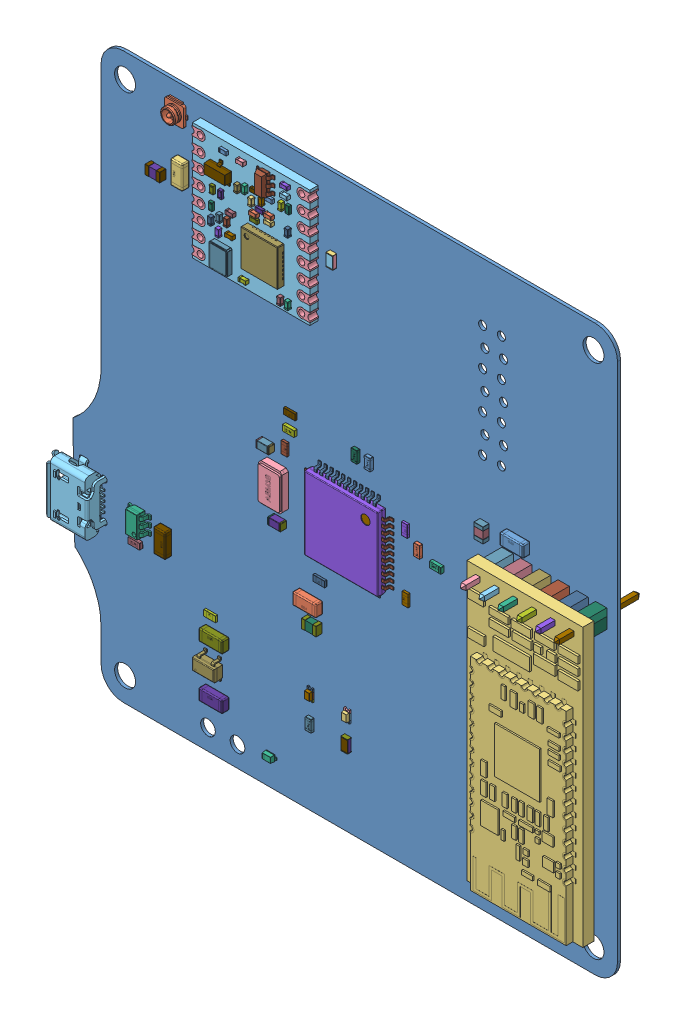
SolidWorks assembly Печатная плата Peggy Receiver, configuration Default. Lengths in mm.
Overall size (75.31 78.06 11.44).
265 component instances, 108 part files, 0 mates.
Components (placement in the parent):
- Печатная плата Peggy Receiver(2)^Печатная плата Peggy Receiver-2: Печатная плата Peggy Receiver(2)^Печатная плата Peggy Receiver [Default] at origin size (75.31 78.06 11.44) (virtual)
  - Board^Печатная плата Peggy Receiver(2)_Печатная плата Peggy Receiver-2: Board^Печатная плата Peggy Receiver(2)_Печатная плата Peggy Receiver [Default] at origin size (73.81 76.5 0.41) (virtual)
    - Open CASCADE STEP translator 7.5 1.1.1^Board_Печатная плата Peggy Receiver(2)_Печатная плата Peggy Receiver-1: Open CASCADE STEP translator 7.5 1.1.1^Board_Печатная плата Peggy Receiver(2)_Печатная плата Peggy Receiver [Default] at (0 0 -0.4115) size (73.81 76.5 0.41) (virtual)
  - XW1^Печатная плата Peggy Receiver(2)_Печатная плата Peggy Receiver-2: XW1^Печатная плата Peggy Receiver(2)_Печатная плата Peggy Receiver [Default] at origin size (3.01 2.86 1.29) (virtual)
    - IPX^XW1_Печатная плата Peggy Receiver(2)_Печатная плата Peggy Receiver-1: IPX^XW1_Печатная плата Peggy Receiver(2)_Печатная плата Peggy Receiver [Default] at (14.0624 73.0251 1.27) x (0 1 0) z (0 0 1) size (3.01 2.86 1.29) (virtual)
  - D1^Печатная плата Peggy Receiver(2)_Печатная плата Peggy Receiver-2: D1^Печатная плата Peggy Receiver(2)_Печатная плата Peggy Receiver [Default] at origin size (15.7 37.6 11.44) (virtual)
    - HC-SERIES^D1_Печатная плата Peggy Receiver(2)_Печатная плата Peggy Receiver-1: HC-SERIES^D1_Печатная плата Peggy Receiver(2)_Печатная плата Peggy Receiver [Default] at (65.255 43.965 4) x (0 -1 0) z (-1 0 0) size (37.6 11.44 15.7) (virtual)
      - HC-SERIES.stp^HC-SERIES_D1_Печатная плата Peggy Receiver(2)_Печатная плата Peggy Receiver-1: HC-SERIES.stp^HC-SERIES_D1_Печатная плата Peggy Receiver(2)_Печатная плата Peggy Receiver [Default] at origin size (37.6 11.44 15.7) (virtual)
        - Assembly1.stp^HC-SERIES.stp_HC-SERIES_D1_Печатная плата Peggy Receiver(2)_Печатная плата Peggy Receiver-1: Assembly1.stp^HC-SERIES.stp_HC-SERIES_D1_Печатная плата Peggy Receiver(2)_Печатная плата Peggy Receiver [Default] at origin size (37.6 2.6 15.7) (virtual)
          - _______-________9.stp^Assembly1.stp_HC-SERIES.stp_HC-SERIES_D1_Печатная плата Peggy Receiver(2)_Печатная плата Peggy Receiver-1: _______-________9.stp^Assembly1.stp_HC-SERIES.stp_HC-SERIES_D1_Печатная плата Peggy Receiver(2)_Печатная плата Peggy Receiver [Default] at origin size (37.6 2.6 15.7) (virtual)
        - Assembly8.stp^HC-SERIES.stp_HC-SERIES_D1_Печатная плата Peggy Receiver(2)_Печатная плата Peggy Receiver-1: Assembly8.stp^HC-SERIES.stp_HC-SERIES_D1_Печатная плата Peggy Receiver(2)_Печатная плата Peggy Receiver [Default] at origin size (2.54 11.44 15.24) (virtual)
          - Pin Header 6 x 1 TH 2.54mm Pitch.stp^Assembly8.stp_HC-SERIES.stp_HC-SERIES_D1_Печатная плата Peggy Receiver(2)_Печатная плата Peggy Receiver-1: Pin Header 6 x 1 TH 2.54mm Pitch.stp^Assembly8.stp_HC-SERIES.stp_HC-SERIES_D1_Печатная плата Peggy Receiver(2)_Печатная плата Peggy Receiver [Default] at (1.3634 -4.0367 -6.3335) x (1 0 0) z (0 -1 0) size (0.64 0.64 11.43) (virtual)
          - Pin Header 6 x 1 TH 2.54mm Pitch-0.stp^Assembly8.stp_HC-SERIES.stp_HC-SERIES_D1_Печатная плата Peggy Receiver(2)_Печатная плата Peggy Receiver-1: Pin Header 6 x 1 TH 2.54mm Pitch-0.stp^Assembly8.stp_HC-SERIES.stp_HC-SERIES_D1_Печатная плата Peggy Receiver(2)_Печатная плата Peggy Receiver [Default] at (1.3634 -4.0367 -6.3335) x (1 0 0) z (0 -1 0) size (0.64 0.64 11.43) (virtual)
          - Pin Header 6 x 1 TH 2.54mm Pitch-1.stp^Assembly8.stp_HC-SERIES.stp_HC-SERIES_D1_Печатная плата Peggy Receiver(2)_Печатная плата Peggy Receiver-1: Pin Header 6 x 1 TH 2.54mm Pitch-1.stp^Assembly8.stp_HC-SERIES.stp_HC-SERIES_D1_Печатная плата Peggy Receiver(2)_Печатная плата Peggy Receiver [Default] at (1.3634 -4.0414 -6.3335) x (1 0 0) z (0 -1 0) size (0.64 0.64 11.43) (virtual)
          - Pin Header 6 x 1 TH 2.54mm Pitch-2.stp^Assembly8.stp_HC-SERIES.stp_HC-SERIES_D1_Печатная плата Peggy Receiver(2)_Печатная плата Peggy Receiver-1: Pin Header 6 x 1 TH 2.54mm Pitch-2.stp^Assembly8.stp_HC-SERIES.stp_HC-SERIES_D1_Печатная плата Peggy Receiver(2)_Печатная плата Peggy Receiver [Default] at (1.3634 -4.0354 -6.3335) x (1 0 0) z (0 -1 0) size (0.64 0.64 11.43) (virtual)
          - Pin Header 6 x 1 TH 2.54mm Pitch-3.stp^Assembly8.stp_HC-SERIES.stp_HC-SERIES_D1_Печатная плата Peggy Receiver(2)_Печатная плата Peggy Receiver-1: Pin Header 6 x 1 TH 2.54mm Pitch-3.stp^Assembly8.stp_HC-SERIES.stp_HC-SERIES_D1_Печатная плата Peggy Receiver(2)_Печатная плата Peggy Receiver [Default] at (1.3634 -4.0354 -6.3335) x (1 0 0) z (0 -1 0) size (0.64 0.63 11.43) (virtual)
          - Pin Header 6 x 1 TH 2.54mm Pitch-4.stp^Assembly8.stp_HC-SERIES.stp_HC-SERIES_D1_Печатная плата Peggy Receiver(2)_Печатная плата Peggy Receiver-1: Pin Header 6 x 1 TH 2.54mm Pitch-4.stp^Assembly8.stp_HC-SERIES.stp_HC-SERIES_D1_Печатная плата Peggy Receiver(2)_Печатная плата Peggy Receiver [Default] at (1.3634 -4.0354 -6.3335) x (1 0 0) z (0 -1 0) size (0.64 0.64 11.43) (virtual)
          - Pin Header 6 x 1 TH 2.54mm Pitch-5.stp^Assembly8.stp_HC-SERIES.stp_HC-SERIES_D1_Печатная плата Peggy Receiver(2)_Печатная плата Peggy Receiver-1: Pin Header 6 x 1 TH 2.54mm Pitch-5.stp^Assembly8.stp_HC-SERIES.stp_HC-SERIES_D1_Печатная плата Peggy Receiver(2)_Печатная плата Peggy Receiver [Default] at (1.3634 -1.5 -6.3335) x (1 0 0) z (0 -1 0) size (2.54 2.54 2.54) (virtual)
          - Pin Header 6 x 1 TH 2.54mm Pitch-6.stp^Assembly8.stp_HC-SERIES.stp_HC-SERIES_D1_Печатная плата Peggy Receiver(2)_Печатная плата Peggy Receiver-1: Pin Header 6 x 1 TH 2.54mm Pitch-6.stp^Assembly8.stp_HC-SERIES.stp_HC-SERIES_D1_Печатная плата Peggy Receiver(2)_Печатная плата Peggy Receiver [Default] at (1.3634 -1.5 -6.3335) x (1 0 0) z (0 -1 0) size (2.54 2.54 2.54) (virtual)
          - Pin Header 6 x 1 TH 2.54mm Pitch-7.stp^Assembly8.stp_HC-SERIES.stp_HC-SERIES_D1_Печатная плата Peggy Receiver(2)_Печатная плата Peggy Receiver-1: Pin Header 6 x 1 TH 2.54mm Pitch-7.stp^Assembly8.stp_HC-SERIES.stp_HC-SERIES_D1_Печатная плата Peggy Receiver(2)_Печатная плата Peggy Receiver [Default] at (1.3634 -1.5 -6.3335) x (1 0 0) z (0 -1 0) size (2.54 2.54 2.54) (virtual)
          - Pin Header 6 x 1 TH 2.54mm Pitch-8.stp^Assembly8.stp_HC-SERIES.stp_HC-SERIES_D1_Печатная плата Peggy Receiver(2)_Печатная плата Peggy Receiver-1: Pin Header 6 x 1 TH 2.54mm Pitch-8.stp^Assembly8.stp_HC-SERIES.stp_HC-SERIES_D1_Печатная плата Peggy Receiver(2)_Печатная плата Peggy Receiver [Default] at (1.3634 -1.5 -6.3335) x (1 0 0) z (0 -1 0) size (2.54 2.54 2.54) (virtual)
          - Pin Header 6 x 1 TH 2.54mm Pitch-9.stp^Assembly8.stp_HC-SERIES.stp_HC-SERIES_D1_Печатная плата Peggy Receiver(2)_Печатная плата Peggy Receiver-1: Pin Header 6 x 1 TH 2.54mm Pitch-9.stp^Assembly8.stp_HC-SERIES.stp_HC-SERIES_D1_Печатная плата Peggy Receiver(2)_Печатная плата Peggy Receiver [Default] at (1.3634 -1.5 -6.3335) x (1 0 0) z (0 -1 0) size (2.54 2.54 2.54) (virtual)
          - Pin Header 6 x 1 TH 2.54mm Pitch-10.stp^Assembly8.stp_HC-SERIES.stp_HC-SERIES_D1_Печатная плата Peggy Receiver(2)_Печатная плата Peggy Receiver-1: Pin Header 6 x 1 TH 2.54mm Pitch-10.stp^Assembly8.stp_HC-SERIES.stp_HC-SERIES_D1_Печатная плата Peggy Receiver(2)_Печатная плата Peggy Receiver [Default] at (1.3634 -1.5 -6.3335) x (1 0 0) z (0 -1 0) size (2.54 2.54 2.54) (virtual)
  - C13^Печатная плата Peggy Receiver(2)_Печатная плата Peggy Receiver-2: C13^Печатная плата Peggy Receiver(2)_Печатная плата Peggy Receiver [Default] at origin size (3.2 1.6 1) (virtual)
    - SW3dPS-1206 SMD Capacitor^C13_Печатная плата Peggy Receiver(2)_Печатная плата Peggy Receiver-1: SW3dPS-1206 SMD Capacitor^C13_Печатная плата Peggy Receiver(2)_Печатная плата Peggy Receiver [Default] at (19.609 14.0729 0) x (1 0 0) z (0 -1 0) size (3.2 1 1.6) (virtual)
  - C12^Печатная плата Peggy Receiver(2)_Печатная плата Peggy Receiver-2: C12^Печатная плата Peggy Receiver(2)_Печатная плата Peggy Receiver [Default] at origin size (3.2 1.6 1) (virtual)
    - SW3dPS-1206 SMD Capacitor^C12_Печатная плата Peggy Receiver(2)_Печатная плата Peggy Receiver-1: SW3dPS-1206 SMD Capacitor^C12_Печатная плата Peggy Receiver(2)_Печатная плата Peggy Receiver [Default] at (19.609 7.0729 0) x (1 0 0) z (0 -1 0) size (3.2 1 1.6) (virtual)
  - C11^Печатная плата Peggy Receiver(2)_Печатная плата Peggy Receiver-2: C11^Печатная плата Peggy Receiver(2)_Печатная плата Peggy Receiver [Default] at origin size (1.6 3.2 1) (virtual)
    - SW3dPS-1206 SMD Capacitor^C11_Печатная плата Peggy Receiver(2)_Печатная плата Peggy Receiver-1: SW3dPS-1206 SMD Capacitor^C11_Печатная плата Peggy Receiver(2)_Печатная плата Peggy Receiver [Default] at (12.6729 22.091 0) x (0 -1 0) z (-1 0 0) size (3.2 1 1.6) (virtual)
  - C6^Печатная плата Peggy Receiver(2)_Печатная плата Peggy Receiver-2: C6^Печатная плата Peggy Receiver(2)_Печатная плата Peggy Receiver [Default] at origin size (3.2 1.6 1) (virtual)
    - SW3dPS-1206 SMD Capacitor^C6_Печатная плата Peggy Receiver(2)_Печатная плата Peggy Receiver-1: SW3dPS-1206 SMD Capacitor^C6_Печатная плата Peggy Receiver(2)_Печатная плата Peggy Receiver [Default] at (60.4 45.7 0) x (1 0 0) z (0 -1 0) size (3.2 1 1.6) (virtual)
  - C5^Печатная плата Peggy Receiver(2)_Печатная плата Peggy Receiver-2: C5^Печатная плата Peggy Receiver(2)_Печатная плата Peggy Receiver [Default] at origin size (3.2 1.6 1) (virtual)
    - SW3dPS-1206 SMD Capacitor^C5_Печатная плата Peggy Receiver(2)_Печатная плата Peggy Receiver-1: SW3dPS-1206 SMD Capacitor^C5_Печатная плата Peggy Receiver(2)_Печатная плата Peggy Receiver [Default] at (32.309 24.6729 0) x (-1 0 0) z (0 1 0) size (3.2 1 1.6) (virtual)
  - C4^Печатная плата Peggy Receiver(2)_Печатная плата Peggy Receiver-2: C4^Печатная плата Peggy Receiver(2)_Печатная плата Peggy Receiver [Default] at origin size (1.6 3.2 1) (virtual)
    - SW3dPS-1206 SMD Capacitor^C4_Печатная плата Peggy Receiver(2)_Печатная плата Peggy Receiver-1: SW3dPS-1206 SMD Capacitor^C4_Печатная плата Peggy Receiver(2)_Печатная плата Peggy Receiver [Default] at (15 66.5 0) x (0 1 0) z (1 0 0) size (3.2 1 1.6) (virtual)
  - ZQ1^Печатная плата Peggy Receiver(2)_Печатная плата Peggy Receiver-2: ZQ1^Печатная плата Peggy Receiver(2)_Печатная плата Peggy Receiver [Default] at origin size (3.18 5 1.11) (virtual)
    - ABM3B^ZQ1_Печатная плата Peggy Receiver(2)_Печатная плата Peggy Receiver-1: ABM3B^ZQ1_Печатная плата Peggy Receiver(2)_Печатная плата Peggy Receiver [Default] at (27.6091 36.0728 0) x (0 1 0) z (1 0 0) size (5 1.11 3.17) (virtual)
  - X2^Печатная плата Peggy Receiver(2)_Печатная плата Peggy Receiver-2: X2^Печатная плата Peggy Receiver(2)_Печатная плата Peggy Receiver [Default] at origin size (5.43 8.2 3.3) (virtual)
    - User Library-MicroUSB-B_Molex_105017-0001^X2_Печатная плата Peggy Receiver(2)_Печатная плата Peggy Receiver-1: User Library-MicroUSB-B_Molex_105017-0001^X2_Печатная плата Peggy Receiver(2)_Печатная плата Peggy Receiver [Default] at (1.7 22.4 1.2) x (0 -1 0) z (-1 0 0) size (8.2 3.3 5.43) (virtual)
  - VD2^Печатная плата Peggy Receiver(2)_Печатная плата Peggy Receiver-2: VD2^Печатная плата Peggy Receiver(2)_Печатная плата Peggy Receiver [Default] at origin size (1.65 0.8 0.65) (virtual)
    - User Library-SOD523-2^VD2_Печатная плата Peggy Receiver(2)_Печатная плата Peggy Receiver-1: User Library-SOD523-2^VD2_Печатная плата Peggy Receiver(2)_Печатная плата Peggy Receiver [Default] at (26.8499 3.7999 0) x (0 1 0) z (1 0 0) size (0.8 0.65 1.65) (virtual)
  - VD1^Печатная плата Peggy Receiver(2)_Печатная плата Peggy Receiver-2: VD1^Печатная плата Peggy Receiver(2)_Печатная плата Peggy Receiver [Default] at origin size (0.81 1.61 0.61) (virtual)
    - User Library-LED_0603_R^VD1_Печатная плата Peggy Receiver(2)_Печатная плата Peggy Receiver-1: User Library-LED_0603_R^VD1_Печатная плата Peggy Receiver(2)_Печатная плата Peggy Receiver [Default] at (32.2999 13.773 0) x (0 1 0) z (0 0 1) size (1.61 0.81 0.61) (virtual)
      - User Library-LED_0603_R_Pocket002^User Library-LED_0603_R_VD1_Печатная плата Peggy Receiver(2)_Печатная плата Peggy Receiver-1: User Library-LED_0603_R_Pocket002^User Library-LED_0603_R_VD1_Печатная плата Peggy Receiver(2)_Печатная плата Peggy Receiver [Default] at origin size (0.41 0.81 0.21) (virtual)
      - User Library-LED_0603_R_Pad004^User Library-LED_0603_R_VD1_Печатная плата Peggy Receiver(2)_Печатная плата Peggy Receiver-1: User Library-LED_0603_R_Pad004^User Library-LED_0603_R_VD1_Печатная плата Peggy Receiver(2)_Печатная плата Peggy Receiver [Default] x (1 0 0) z (0 0 -1) size (0.4 0.8 0) (virtual)
      - User Library-LED_0603_R_Fillet^User Library-LED_0603_R_VD1_Печатная плата Peggy Receiver(2)_Печатная плата Peggy Receiver-1: User Library-LED_0603_R_Fillet^User Library-LED_0603_R_VD1_Печатная плата Peggy Receiver(2)_Печатная плата Peggy Receiver [Default] at origin size (1 0.7 0.4) (virtual)
      - User Library-LED_0603_R_Pocket001^User Library-LED_0603_R_VD1_Печатная плата Peggy Receiver(2)_Печатная плата Peggy Receiver-1: User Library-LED_0603_R_Pocket001^User Library-LED_0603_R_VD1_Печатная плата Peggy Receiver(2)_Печатная плата Peggy Receiver [Default] at origin size (0.4 0.8 0.2) (virtual)
      - User Library-LED_0603_R_Pad^User Library-LED_0603_R_VD1_Печатная плата Peggy Receiver(2)_Печатная плата Peggy Receiver-1: User Library-LED_0603_R_Pad^User Library-LED_0603_R_VD1_Печатная плата Peggy Receiver(2)_Печатная плата Peggy Receiver [Default] at origin size (0.8 0.8 0.2) (virtual)
  - U1^Печатная плата Peggy Receiver(2)_Печатная плата Peggy Receiver-2: U1^Печатная плата Peggy Receiver(2)_Печатная плата Peggy Receiver [Default] at origin size (3 2.8 1.4) (virtual)
    - AP2112K-3.3TRG1--3DModel-STEP-1^U1_Печатная плата Peggy Receiver(2)_Печатная плата Peggy Receiver-1: AP2112K-3.3TRG1--3DModel-STEP-1^U1_Печатная плата Peggy Receiver(2)_Печатная плата Peggy Receiver [Default] at (19.009 10.5729 0) x (-1 0 0) z (0 1 0) size (3 1.4 2.8) (virtual)
  - R9^Печатная плата Peggy Receiver(2)_Печатная плата Peggy Receiver-2: R9^Печатная плата Peggy Receiver(2)_Печатная плата Peggy Receiver [Default] at origin size (1.61 0.81 0.46) (virtual)
    - chip_0603_r^R9_Печатная плата Peggy Receiver(2)_Печатная плата Peggy Receiver-1: chip_0603_r^R9_Печатная плата Peggy Receiver(2)_Печатная плата Peggy Receiver [Default] at (9.4728 19.7911 0.21) x (0 1 0) z (0 0 1) size (0.81 1.61 0.46) (virtual)
  - R8^Печатная плата Peggy Receiver(2)_Печатная плата Peggy Receiver-2: R8^Печатная плата Peggy Receiver(2)_Печатная плата Peggy Receiver [Default] at origin size (0.81 1.61 0.46) (virtual)
    - chip_0603_r^R8_Печатная плата Peggy Receiver(2)_Печатная плата Peggy Receiver-1: chip_0603_r^R8_Печатная плата Peggy Receiver(2)_Печатная плата Peggy Receiver [Default] at (32.2999 11.0999 0.21) x (-1 0 0) z (0 0 1) size (0.81 1.61 0.46) (virtual)
  - R7^Печатная плата Peggy Receiver(2)_Печатная плата Peggy Receiver-2: R7^Печатная плата Peggy Receiver(2)_Печатная плата Peggy Receiver [Default] at origin size (0.81 1.61 0.46) (virtual)
    - chip_0603_r^R7_Печатная плата Peggy Receiver(2)_Печатная плата Peggy Receiver-1: chip_0603_r^R7_Печатная плата Peggy Receiver(2)_Печатная плата Peggy Receiver [Default] at (38.5089 45.7728 0.21) x (-1 0 0) z (0 0 1) size (0.81 1.61 0.46) (virtual)
  - R6^Печатная плата Peggy Receiver(2)_Печатная плата Peggy Receiver-2: R6^Печатная плата Peggy Receiver(2)_Печатная плата Peggy Receiver [Default] at origin size (0.9 1.7 0.55) (virtual)
    - 6665909488^R6_Печатная плата Peggy Receiver(2)_Печатная плата Peggy Receiver-1: 6665909488^R6_Печатная плата Peggy Receiver(2)_Печатная плата Peggy Receiver [Default] at (37.2999 10.5001 0) x (0 1 0) z (0 0 1) size (1.7 0.9 0.55) (virtual)
      - Terminal^6665909488_R6_Печатная плата Peggy Receiver(2)_Печатная плата Peggy Receiver-1: Terminal^6665909488_R6_Печатная плата Peggy Receiver(2)_Печатная плата Peggy Receiver [Default] at (-0.85 -0.45 0) size (0.1 0.9 0.55) (virtual)
        - Open CASCADE STEP translator 6.8 15.2.1^Terminal_6665909488_R6_Печатная плата Peggy Receiver(2)_Печатная плата Peggy Receiver-1: Open CASCADE STEP translator 6.8 15.2.1^Terminal_6665909488_R6_Печатная плата Peggy Receiver(2)_Печатная плата Peggy Receiver [Default] at origin size (0.1 0.9 0.55) (virtual)
      - Terminal^6665909488_R6_Печатная плата Peggy Receiver(2)_Печатная плата Peggy Receiver-2: Terminal^6665909488_R6_Печатная плата Peggy Receiver(2)_Печатная плата Peggy Receiver [Default] at (0.85 0.45 0) x (-1 0 0) z (0 0 1) size (0.1 0.9 0.55) (virtual)
        - Open CASCADE STEP translator 6.8 15.2.1^Terminal_6665909488_R6_Печатная плата Peggy Receiver(2)_Печатная плата Peggy Receiver-1: Open CASCADE STEP translator 6.8 15.2.1^Terminal_6665909488_R6_Печатная плата Peggy Receiver(2)_Печатная плата Peggy Receiver [Default] at origin size (0.1 0.9 0.55) (virtual)
      - Mid_Body^6665909488_R6_Печатная плата Peggy Receiver(2)_Печатная плата Peggy Receiver-1: Mid_Body^6665909488_R6_Печатная плата Peggy Receiver(2)_Печатная плата Peggy Receiver [Default] at (-0.85 -0.45 0) size (1.59 0.9 0.44) (virtual)
      - Mark^6665909488_R6_Печатная плата Peggy Receiver(2)_Печатная плата Peggy Receiver-1: Mark^6665909488_R6_Печатная плата Peggy Receiver(2)_Печатная плата Peggy Receiver [Default] at (-0.75 -0.45 0.495) size (1.5 0.9 0.06) (virtual)
  - R5^Печатная плата Peggy Receiver(2)_Печатная плата Peggy Receiver-2: R5^Печатная плата Peggy Receiver(2)_Печатная плата Peggy Receiver [Default] at origin size (0.81 1.61 0.46) (virtual)
    - chip_0603_r^R5_Печатная плата Peggy Receiver(2)_Печатная плата Peggy Receiver-1: chip_0603_r^R5_Печатная плата Peggy Receiver(2)_Печатная плата Peggy Receiver [Default] at (40.3089 45.7728 0.21) x (-1 0 0) z (0 0 1) size (0.81 1.61 0.46) (virtual)
  - R4^Печатная плата Peggy Receiver(2)_Печатная плата Peggy Receiver-2: R4^Печатная плата Peggy Receiver(2)_Печатная плата Peggy Receiver [Default] at origin size (0.81 1.61 0.46) (virtual)
    - chip_0603_r^R4_Печатная плата Peggy Receiver(2)_Печатная плата Peggy Receiver-1: chip_0603_r^R4_Печатная плата Peggy Receiver(2)_Печатная плата Peggy Receiver [Default] at (47.0089 38.8728 0.21) x (-1 0 0) z (0 0 1) size (0.81 1.61 0.46) (virtual)
  - R3^Печатная плата Peggy Receiver(2)_Печатная плата Peggy Receiver-2: R3^Печатная плата Peggy Receiver(2)_Печатная плата Peggy Receiver [Default] at origin size (0.9 1.7 0.55) (virtual)
    - 6665909808^R3_Печатная плата Peggy Receiver(2)_Печатная плата Peggy Receiver-1: 6665909808^R3_Печатная плата Peggy Receiver(2)_Печатная плата Peggy Receiver [Default] at (35.3001 66.2999 0) x (0 -1 0) z (0 0 1) size (1.7 0.9 0.55) (virtual)
      - Terminal-1^6665909808_R3_Печатная плата Peggy Receiver(2)_Печатная плата Peggy Receiver-1: Terminal-1^6665909808_R3_Печатная плата Peggy Receiver(2)_Печатная плата Peggy Receiver [Default] at (-0.85 -0.45 0) size (0.1 0.9 0.55) (virtual)
        - Open CASCADE STEP translator 6.8 15.2.1-0^Terminal-1_6665909808_R3_Печатная плата Peggy Receiver(2)_Печатная плата Peggy Receiver-1: Open CASCADE STEP translator 6.8 15.2.1-0^Terminal-1_6665909808_R3_Печатная плата Peggy Receiver(2)_Печатная плата Peggy Receiver [Default] at origin size (0.1 0.9 0.55) (virtual)
      - Terminal-1^6665909808_R3_Печатная плата Peggy Receiver(2)_Печатная плата Peggy Receiver-2: Terminal-1^6665909808_R3_Печатная плата Peggy Receiver(2)_Печатная плата Peggy Receiver [Default] at (0.85 0.45 0) x (-1 0 0) z (0 0 1) size (0.1 0.9 0.55) (virtual)
        - Open CASCADE STEP translator 6.8 15.2.1-0^Terminal-1_6665909808_R3_Печатная плата Peggy Receiver(2)_Печатная плата Peggy Receiver-1: Open CASCADE STEP translator 6.8 15.2.1-0^Terminal-1_6665909808_R3_Печатная плата Peggy Receiver(2)_Печатная плата Peggy Receiver [Default] at origin size (0.1 0.9 0.55) (virtual)
      - Mid_Body-1^6665909808_R3_Печатная плата Peggy Receiver(2)_Печатная плата Peggy Receiver-1: Mid_Body-1^6665909808_R3_Печатная плата Peggy Receiver(2)_Печатная плата Peggy Receiver [Default] at (-0.85 -0.45 0) size (1.59 0.9 0.44) (virtual)
      - Mark-2^6665909808_R3_Печатная плата Peggy Receiver(2)_Печатная плата Peggy Receiver-1: Mark-2^6665909808_R3_Печатная плата Peggy Receiver(2)_Печатная плата Peggy Receiver [Default] at (-0.75 -0.45 0.495) size (1.5 0.9 0.06) (virtual)
  - R2^Печатная плата Peggy Receiver(2)_Печатная плата Peggy Receiver-2: R2^Печатная плата Peggy Receiver(2)_Печатная плата Peggy Receiver [Default] at origin size (1.61 0.81 0.46) (virtual)
    - chip_0603_r^R2_Печатная плата Peggy Receiver(2)_Печатная плата Peggy Receiver-1: chip_0603_r^R2_Печатная плата Peggy Receiver(2)_Печатная плата Peggy Receiver [Default] at (48.7091 37.3728 0.21) x (0 -1 0) z (0 0 1) size (0.81 1.61 0.46) (virtual)
  - R1^Печатная плата Peggy Receiver(2)_Печатная плата Peggy Receiver-2: R1^Печатная плата Peggy Receiver(2)_Печатная плата Peggy Receiver [Default] at origin size (1.61 0.81 0.46) (virtual)
    - chip_0603_r^R1_Печатная плата Peggy Receiver(2)_Печатная плата Peggy Receiver-1: chip_0603_r^R1_Печатная плата Peggy Receiver(2)_Печатная плата Peggy Receiver [Default] at (30.4089 43.473 0.21) x (0 1 0) z (0 0 1) size (0.81 1.61 0.46) (virtual)
  - MPU1^Печатная плата Peggy Receiver(2)_Печатная плата Peggy Receiver-2: MPU1^Печатная плата Peggy Receiver(2)_Печатная плата Peggy Receiver [Default] at origin size (14.96 12 1.2) (virtual)
    - 6665910048^MPU1_Печатная плата Peggy Receiver(2)_Печатная плата Peggy Receiver-1: 6665910048^MPU1_Печатная плата Peggy Receiver(2)_Печатная плата Peggy Receiver [Default] at (37.5091 35.7228 0) x (0 -1 0) z (0 0 1) size (12 14.96 1.2) (virtual)
      - Body^6665910048_MPU1_Печатная плата Peggy Receiver(2)_Печатная плата Peggy Receiver-1: Body^6665910048_MPU1_Печатная плата Peggy Receiver(2)_Печатная плата Peggy Receiver [Default] at (-5 -5 0) size (10.01 10.01 1.15) (virtual)
        - Open CASCADE STEP translator 6.8 62.2.1^Body_6665910048_MPU1_Печатная плата Peggy Receiver(2)_Печатная плата Peggy Receiver-1: Open CASCADE STEP translator 6.8 62.2.1^Body_6665910048_MPU1_Печатная плата Peggy Receiver(2)_Печатная плата Peggy Receiver [Default] at origin size (10.01 10.01 1.15) (virtual)
      - Open CASCADE STEP translator 6.8 62.1^6665910048_MPU1_Печатная плата Peggy Receiver(2)_Печатная плата Peggy Receiver-1: Open CASCADE STEP translator 6.8 62.1^6665910048_MPU1_Печатная плата Peggy Receiver(2)_Печатная плата Peggy Receiver [Default] at (-5 -5 0.001) size (1.26 1.26 0.01) (virtual)
      - Leader^6665910048_MPU1_Печатная плата Peggy Receiver(2)_Печатная плата Peggy Receiver-1: Leader^6665910048_MPU1_Печатная плата Peggy Receiver(2)_Печатная плата Peggy Receiver [Default] at (-5 -4 0) x (-1 0 0) z (0 0 1) size (1 0.38 0.68) (virtual)
      - Leader^6665910048_MPU1_Печатная плата Peggy Receiver(2)_Печатная плата Peggy Receiver-2: Leader^6665910048_MPU1_Печатная плата Peggy Receiver(2)_Печатная плата Peggy Receiver [Default] at (-5 -3.2 0) x (-1 0 0) z (0 0 1) size (1 0.38 0.68) (virtual)
      - Leader^6665910048_MPU1_Печатная плата Peggy Receiver(2)_Печатная плата Peggy Receiver-3: Leader^6665910048_MPU1_Печатная плата Peggy Receiver(2)_Печатная плата Peggy Receiver [Default] at (-5 -2.4 0) x (-1 0 0) z (0 0 1) size (1 0.38 0.68) (virtual)
      - Leader^6665910048_MPU1_Печатная плата Peggy Receiver(2)_Печатная плата Peggy Receiver-4: Leader^6665910048_MPU1_Печатная плата Peggy Receiver(2)_Печатная плата Peggy Receiver [Default] at (-5 -1.6 0) x (-1 0 0) z (0 0 1) size (1 0.38 0.68) (virtual)
      - Leader^6665910048_MPU1_Печатная плата Peggy Receiver(2)_Печатная плата Peggy Receiver-5: Leader^6665910048_MPU1_Печатная плата Peggy Receiver(2)_Печатная плата Peggy Receiver [Default] at (-5 -0.8 0) x (-1 0 0) z (0 0 1) size (1 0.38 0.68) (virtual)
      - Leader^6665910048_MPU1_Печатная плата Peggy Receiver(2)_Печатная плата Peggy Receiver-6: Leader^6665910048_MPU1_Печатная плата Peggy Receiver(2)_Печатная плата Peggy Receiver [Default] at (-5 0 0) x (-1 0 0) z (0 0 1) size (1 0.38 0.68) (virtual)
      - Leader^6665910048_MPU1_Печатная плата Peggy Receiver(2)_Печатная плата Peggy Receiver-7: Leader^6665910048_MPU1_Печатная плата Peggy Receiver(2)_Печатная плата Peggy Receiver [Default] at (-5 0.8 0) x (-1 0 0) z (0 0 1) size (1 0.38 0.68) (virtual)
      - Leader^6665910048_MPU1_Печатная плата Peggy Receiver(2)_Печатная плата Peggy Receiver-8: Leader^6665910048_MPU1_Печатная плата Peggy Receiver(2)_Печатная плата Peggy Receiver [Default] at (-5 1.6 0) x (-1 0 0) z (0 0 1) size (1 0.38 0.68) (virtual)
      - Leader^6665910048_MPU1_Печатная плата Peggy Receiver(2)_Печатная плата Peggy Receiver-9: Leader^6665910048_MPU1_Печатная плата Peggy Receiver(2)_Печатная плата Peggy Receiver [Default] at (-5 2.4 0) x (-1 0 0) z (0 0 1) size (1 0.38 0.68) (virtual)
      - Leader^6665910048_MPU1_Печатная плата Peggy Receiver(2)_Печатная плата Peggy Receiver-10: Leader^6665910048_MPU1_Печатная плата Peggy Receiver(2)_Печатная плата Peggy Receiver [Default] at (-5 3.2 0) x (-1 0 0) z (0 0 1) size (1 0.38 0.68) (virtual)
      - Leader^6665910048_MPU1_Печатная плата Peggy Receiver(2)_Печатная плата Peggy Receiver-11: Leader^6665910048_MPU1_Печатная плата Peggy Receiver(2)_Печатная плата Peggy Receiver [Default] at (-5 4 0) x (-1 0 0) z (0 0 1) size (1 0.38 0.68) (virtual)
      - Leader^6665910048_MPU1_Печатная плата Peggy Receiver(2)_Печатная плата Peggy Receiver-12: Leader^6665910048_MPU1_Печатная плата Peggy Receiver(2)_Печатная плата Peggy Receiver [Default] at (5 -4 0) size (1 0.38 0.68) (virtual)
      - Leader^6665910048_MPU1_Печатная плата Peggy Receiver(2)_Печатная плата Peggy Receiver-13: Leader^6665910048_MPU1_Печатная плата Peggy Receiver(2)_Печатная плата Peggy Receiver [Default] at (5 -3.2 0) size (1 0.38 0.68) (virtual)
      - Leader^6665910048_MPU1_Печатная плата Peggy Receiver(2)_Печатная плата Peggy Receiver-14: Leader^6665910048_MPU1_Печатная плата Peggy Receiver(2)_Печатная плата Peggy Receiver [Default] at (5 -2.4 0) size (1 0.38 0.68) (virtual)
      - Leader^6665910048_MPU1_Печатная плата Peggy Receiver(2)_Печатная плата Peggy Receiver-15: Leader^6665910048_MPU1_Печатная плата Peggy Receiver(2)_Печатная плата Peggy Receiver [Default] at (5 -1.6 0) size (1 0.38 0.68) (virtual)
      - Leader^6665910048_MPU1_Печатная плата Peggy Receiver(2)_Печатная плата Peggy Receiver-16: Leader^6665910048_MPU1_Печатная плата Peggy Receiver(2)_Печатная плата Peggy Receiver [Default] at (5 -0.8 0) size (1 0.38 0.68) (virtual)
      - Leader^6665910048_MPU1_Печатная плата Peggy Receiver(2)_Печатная плата Peggy Receiver-17: Leader^6665910048_MPU1_Печатная плата Peggy Receiver(2)_Печатная плата Peggy Receiver [Default] at (5 0 0) size (1 0.38 0.68) (virtual)
      - Leader^6665910048_MPU1_Печатная плата Peggy Receiver(2)_Печатная плата Peggy Receiver-18: Leader^6665910048_MPU1_Печатная плата Peggy Receiver(2)_Печатная плата Peggy Receiver [Default] at (5 0.8 0) size (1 0.38 0.68) (virtual)
      - Leader^6665910048_MPU1_Печатная плата Peggy Receiver(2)_Печатная плата Peggy Receiver-19: Leader^6665910048_MPU1_Печатная плата Peggy Receiver(2)_Печатная плата Peggy Receiver [Default] at (5 1.6 0) size (1 0.38 0.68) (virtual)
      - Leader^6665910048_MPU1_Печатная плата Peggy Receiver(2)_Печатная плата Peggy Receiver-20: Leader^6665910048_MPU1_Печатная плата Peggy Receiver(2)_Печатная плата Peggy Receiver [Default] at (5 2.4 0) size (1 0.38 0.68) (virtual)
      - Leader^6665910048_MPU1_Печатная плата Peggy Receiver(2)_Печатная плата Peggy Receiver-21: Leader^6665910048_MPU1_Печатная плата Peggy Receiver(2)_Печатная плата Peggy Receiver [Default] at (5 3.2 0) size (1 0.38 0.68) (virtual)
      - Leader^6665910048_MPU1_Печатная плата Peggy Receiver(2)_Печатная плата Peggy Receiver-22: Leader^6665910048_MPU1_Печатная плата Peggy Receiver(2)_Печатная плата Peggy Receiver [Default] at (5 4 0) size (1 0.38 0.68) (virtual)
      - Leader-3^6665910048_MPU1_Печатная плата Peggy Receiver(2)_Печатная плата Peggy Receiver-1: Leader-3^6665910048_MPU1_Печатная плата Peggy Receiver(2)_Печатная плата Peggy Receiver [Default] at (-4 -5 0) x (0 -1 0) z (0 0 1) size (1 0.38 0.68) (virtual)
      - Leader-3^6665910048_MPU1_Печатная плата Peggy Receiver(2)_Печатная плата Peggy Receiver-2: Leader-3^6665910048_MPU1_Печатная плата Peggy Receiver(2)_Печатная плата Peggy Receiver [Default] at (-3.2 -5 0) x (0 -1 0) z (0 0 1) size (1 0.38 0.68) (virtual)
      - Leader-3^6665910048_MPU1_Печатная плата Peggy Receiver(2)_Печатная плата Peggy Receiver-3: Leader-3^6665910048_MPU1_Печатная плата Peggy Receiver(2)_Печатная плата Peggy Receiver [Default] at (-2.4 -5 0) x (0 -1 0) z (0 0 1) size (1 0.38 0.68) (virtual)
      - Leader-3^6665910048_MPU1_Печатная плата Peggy Receiver(2)_Печатная плата Peggy Receiver-4: Leader-3^6665910048_MPU1_Печатная плата Peggy Receiver(2)_Печатная плата Peggy Receiver [Default] at (-1.6 -5 0) x (0 -1 0) z (0 0 1) size (1 0.38 0.68) (virtual)
      - Leader-3^6665910048_MPU1_Печатная плата Peggy Receiver(2)_Печатная плата Peggy Receiver-5: Leader-3^6665910048_MPU1_Печатная плата Peggy Receiver(2)_Печатная плата Peggy Receiver [Default] at (-0.8 -5 0) x (0 -1 0) z (0 0 1) size (1 0.38 0.68) (virtual)
      - Leader-3^6665910048_MPU1_Печатная плата Peggy Receiver(2)_Печатная плата Peggy Receiver-6: Leader-3^6665910048_MPU1_Печатная плата Peggy Receiver(2)_Печатная плата Peggy Receiver [Default] at (0 -5 0) x (0 -1 0) z (0 0 1) size (1 0.38 0.68) (virtual)
      - Leader-3^6665910048_MPU1_Печатная плата Peggy Receiver(2)_Печатная плата Peggy Receiver-7: Leader-3^6665910048_MPU1_Печатная плата Peggy Receiver(2)_Печатная плата Peggy Receiver [Default] at (0.8 -5 0) x (0 -1 0) z (0 0 1) size (1 0.38 0.68) (virtual)
      - Leader-3^6665910048_MPU1_Печатная плата Peggy Receiver(2)_Печатная плата Peggy Receiver-8: Leader-3^6665910048_MPU1_Печатная плата Peggy Receiver(2)_Печатная плата Peggy Receiver [Default] at (1.6 -5 0) x (0 -1 0) z (0 0 1) size (1 0.38 0.68) (virtual)
      - Leader-3^6665910048_MPU1_Печатная плата Peggy Receiver(2)_Печатная плата Peggy Receiver-9: Leader-3^6665910048_MPU1_Печатная плата Peggy Receiver(2)_Печатная плата Peggy Receiver [Default] at (2.4 -5 0) x (0 -1 0) z (0 0 1) size (1 0.38 0.68) (virtual)
      - Leader-3^6665910048_MPU1_Печатная плата Peggy Receiver(2)_Печатная плата Peggy Receiver-10: Leader-3^6665910048_MPU1_Печатная плата Peggy Receiver(2)_Печатная плата Peggy Receiver [Default] at (3.2 -5 0) x (0 -1 0) z (0 0 1) size (1 0.38 0.68) (virtual)
      - Leader-3^6665910048_MPU1_Печатная плата Peggy Receiver(2)_Печатная плата Peggy Receiver-11: Leader-3^6665910048_MPU1_Печатная плата Peggy Receiver(2)_Печатная плата Peggy Receiver [Default] at (4 -5 0) x (0 -1 0) z (0 0 1) size (1 0.38 0.68) (virtual)
      - Leader-3^6665910048_MPU1_Печатная плата Peggy Receiver(2)_Печатная плата Peggy Receiver-12: Leader-3^6665910048_MPU1_Печатная плата Peggy Receiver(2)_Печатная плата Peggy Receiver [Default] at (-4 5 0) x (0 1 0) z (0 0 1) size (1 0.38 0.68) (virtual)
      - Leader-3^6665910048_MPU1_Печатная плата Peggy Receiver(2)_Печатная плата Peggy Receiver-13: Leader-3^6665910048_MPU1_Печатная плата Peggy Receiver(2)_Печатная плата Peggy Receiver [Default] at (-3.2 5 0) x (0 1 0) z (0 0 1) size (1 0.38 0.68) (virtual)
      - Leader-3^6665910048_MPU1_Печатная плата Peggy Receiver(2)_Печатная плата Peggy Receiver-14: Leader-3^6665910048_MPU1_Печатная плата Peggy Receiver(2)_Печатная плата Peggy Receiver [Default] at (-2.4 5 0) x (0 1 0) z (0 0 1) size (1 0.38 0.68) (virtual)
      - Leader-3^6665910048_MPU1_Печатная плата Peggy Receiver(2)_Печатная плата Peggy Receiver-15: Leader-3^6665910048_MPU1_Печатная плата Peggy Receiver(2)_Печатная плата Peggy Receiver [Default] at (-1.6 5 0) x (0 1 0) z (0 0 1) size (1 0.38 0.68) (virtual)
      - Leader-3^6665910048_MPU1_Печатная плата Peggy Receiver(2)_Печатная плата Peggy Receiver-16: Leader-3^6665910048_MPU1_Печатная плата Peggy Receiver(2)_Печатная плата Peggy Receiver [Default] at (-0.8 5 0) x (0 1 0) z (0 0 1) size (1 0.38 0.68) (virtual)
      - Leader-3^6665910048_MPU1_Печатная плата Peggy Receiver(2)_Печатная плата Peggy Receiver-17: Leader-3^6665910048_MPU1_Печатная плата Peggy Receiver(2)_Печатная плата Peggy Receiver [Default] at (0 5 0) x (0 1 0) z (0 0 1) size (1 0.38 0.68) (virtual)
      - Leader-3^6665910048_MPU1_Печатная плата Peggy Receiver(2)_Печатная плата Peggy Receiver-18: Leader-3^6665910048_MPU1_Печатная плата Peggy Receiver(2)_Печатная плата Peggy Receiver [Default] at (0.8 5 0) x (0 1 0) z (0 0 1) size (1 0.38 0.68) (virtual)
      - Leader-3^6665910048_MPU1_Печатная плата Peggy Receiver(2)_Печатная плата Peggy Receiver-19: Leader-3^6665910048_MPU1_Печатная плата Peggy Receiver(2)_Печатная плата Peggy Receiver [Default] at (1.6 5 0) x (0 1 0) z (0 0 1) size (1 0.38 0.68) (virtual)
      - Leader-3^6665910048_MPU1_Печатная плата Peggy Receiver(2)_Печатная плата Peggy Receiver-20: Leader-3^6665910048_MPU1_Печатная плата Peggy Receiver(2)_Печатная плата Peggy Receiver [Default] at (2.4 5 0) x (0 1 0) z (0 0 1) size (1 0.38 0.68) (virtual)
      - Leader-3^6665910048_MPU1_Печатная плата Peggy Receiver(2)_Печатная плата Peggy Receiver-21: Leader-3^6665910048_MPU1_Печатная плата Peggy Receiver(2)_Печатная плата Peggy Receiver [Default] at (3.2 5 0) x (0 1 0) z (0 0 1) size (1 0.38 0.68) (virtual)
      - Leader-3^6665910048_MPU1_Печатная плата Peggy Receiver(2)_Печатная плата Peggy Receiver-22: Leader-3^6665910048_MPU1_Печатная плата Peggy Receiver(2)_Печатная плата Peggy Receiver [Default] at (4 5 0) x (0 1 0) z (0 0 1) size (1 0.38 0.68) (virtual)
    - User Library-VQFN(44)^MPU1_Печатная плата Peggy Receiver(2)_Печатная плата Peggy Receiver-1: User Library-VQFN(44)^MPU1_Печатная плата Peggy Receiver(2)_Печатная плата Peggy Receiver [Default] at (33.963 32.1998 0) x (1 0 0) z (0 -1 0) size (7.1 0.95 7.1) (virtual)
  - L3^Печатная плата Peggy Receiver(2)_Печатная плата Peggy Receiver-2: L3^Печатная плата Peggy Receiver(2)_Печатная плата Peggy Receiver [Default] at origin size (1.25 2 0.85) (virtual)
    - User Library-FB_2012-1^L3_Печатная плата Peggy Receiver(2)_Печатная плата Peggy Receiver-1: User Library-FB_2012-1^L3_Печатная плата Peggy Receiver(2)_Печатная плата Peggy Receiver [Default] at (55.7999 44.8001 0) x (0 1 0) z (0 0 1) size (2 1.25 0.85) (virtual)
      - User Library-FB_2012-1_Pad001^User Library-FB_2012-1_L3_Печатная плата Peggy Receiver(2)_Печатная плата Peggy Receiver-1: User Library-FB_2012-1_Pad001^User Library-FB_2012-1_L3_Печатная плата Peggy Receiver(2)_Печатная плата Peggy Receiver [Default] at (0 0 0.03) size (1.94 1.19 0.79) (virtual)
      - User Library-FB_2012-1_Cut^User Library-FB_2012-1_L3_Печатная плата Peggy Receiver(2)_Печатная плата Peggy Receiver-1: User Library-FB_2012-1_Cut^User Library-FB_2012-1_L3_Печатная плата Peggy Receiver(2)_Печатная плата Peggy Receiver [Default] at origin size (2 1.25 0.85) (virtual)
  - L2^Печатная плата Peggy Receiver(2)_Печатная плата Peggy Receiver-2: L2^Печатная плата Peggy Receiver(2)_Печатная плата Peggy Receiver [Default] at origin size (2 1.25 0.85) (virtual)
    - User Library-FB_2012-1^L2_Печатная плата Peggy Receiver(2)_Печатная плата Peggy Receiver-1: User Library-FB_2012-1^L2_Печатная плата Peggy Receiver(2)_Печатная плата Peggy Receiver [Default] at (32.8001 22.2001 0) x (1 0 0) z (0 0 1) size (2 1.25 0.85) (virtual)
      - User Library-FB_2012-1_Pad001^User Library-FB_2012-1_L2_Печатная плата Peggy Receiver(2)_Печатная плата Peggy Receiver-1: User Library-FB_2012-1_Pad001^User Library-FB_2012-1_L2_Печатная плата Peggy Receiver(2)_Печатная плата Peggy Receiver [Default] at (0 0 0.03) size (1.94 1.19 0.79) (virtual)
      - User Library-FB_2012-1_Cut^User Library-FB_2012-1_L2_Печатная плата Peggy Receiver(2)_Печатная плата Peggy Receiver-1: User Library-FB_2012-1_Cut^User Library-FB_2012-1_L2_Печатная плата Peggy Receiver(2)_Печатная плата Peggy Receiver [Default] at origin size (2 1.25 0.85) (virtual)
  - L1^Печатная плата Peggy Receiver(2)_Печатная плата Peggy Receiver-2: L1^Печатная плата Peggy Receiver(2)_Печатная плата Peggy Receiver [Default] at origin size (2 1.25 0.85) (virtual)
    - User Library-FB_2012-1^L1_Печатная плата Peggy Receiver(2)_Печатная плата Peggy Receiver-1: User Library-FB_2012-1^L1_Печатная плата Peggy Receiver(2)_Печатная плата Peggy Receiver [Default] at (11.5999 64.8999 0) x (-1 0 0) z (0 0 1) size (2 1.25 0.85) (virtual)
      - User Library-FB_2012-1_Pad001^User Library-FB_2012-1_L1_Печатная плата Peggy Receiver(2)_Печатная плата Peggy Receiver-1: User Library-FB_2012-1_Pad001^User Library-FB_2012-1_L1_Печатная плата Peggy Receiver(2)_Печатная плата Peggy Receiver [Default] at (0 0 0.03) size (1.94 1.19 0.79) (virtual)
      - User Library-FB_2012-1_Cut^User Library-FB_2012-1_L1_Печатная плата Peggy Receiver(2)_Печатная плата Peggy Receiver-1: User Library-FB_2012-1_Cut^User Library-FB_2012-1_L1_Печатная плата Peggy Receiver(2)_Печатная плата Peggy Receiver [Default] at origin size (2 1.25 0.85) (virtual)
  - HL1^Печатная плата Peggy Receiver(2)_Печатная плата Peggy Receiver-2: HL1^Печатная плата Peggy Receiver(2)_Печатная плата Peggy Receiver [Default] at origin size (0.81 1.61 0.61) (virtual)
    - User Library-LED_0603_G^HL1_Печатная плата Peggy Receiver(2)_Печатная плата Peggy Receiver-1: User Library-LED_0603_G^HL1_Печатная плата Peggy Receiver(2)_Печатная плата Peggy Receiver [Default] at (37.2999 13.773 0) x (0 1 0) z (0 0 1) size (1.61 0.81 0.61) (virtual)
      - User Library-LED_0603_G_Pocket002^User Library-LED_0603_G_HL1_Печатная плата Peggy Receiver(2)_Печатная плата Peggy Receiver-1: User Library-LED_0603_G_Pocket002^User Library-LED_0603_G_HL1_Печатная плата Peggy Receiver(2)_Печатная плата Peggy Receiver [Default] at origin size (0.41 0.81 0.21) (virtual)
      - User Library-LED_0603_G_Pad004^User Library-LED_0603_G_HL1_Печатная плата Peggy Receiver(2)_Печатная плата Peggy Receiver-1: User Library-LED_0603_G_Pad004^User Library-LED_0603_G_HL1_Печатная плата Peggy Receiver(2)_Печатная плата Peggy Receiver [Default] x (1 0 0) z (0 0 -1) size (0.4 0.8 0) (virtual)
      - User Library-LED_0603_G_Fillet^User Library-LED_0603_G_HL1_Печатная плата Peggy Receiver(2)_Печатная плата Peggy Receiver-1: User Library-LED_0603_G_Fillet^User Library-LED_0603_G_HL1_Печатная плата Peggy Receiver(2)_Печатная плата Peggy Receiver [Default] at origin size (1 0.7 0.4) (virtual)
      - User Library-LED_0603_G_Pocket001^User Library-LED_0603_G_HL1_Печатная плата Peggy Receiver(2)_Печатная плата Peggy Receiver-1: User Library-LED_0603_G_Pocket001^User Library-LED_0603_G_HL1_Печатная плата Peggy Receiver(2)_Печатная плата Peggy Receiver [Default] at origin size (0.4 0.8 0.2) (virtual)
      - User Library-LED_0603_G_Pad^User Library-LED_0603_G_HL1_Печатная плата Peggy Receiver(2)_Печатная плата Peggy Receiver-1: User Library-LED_0603_G_Pad^User Library-LED_0603_G_HL1_Печатная плата Peggy Receiver(2)_Печатная плата Peggy Receiver [Default] at origin size (0.8 0.8 0.2) (virtual)
  - DD1^Печатная плата Peggy Receiver(2)_Печатная плата Peggy Receiver-2: DD1^Печатная плата Peggy Receiver(2)_Печатная плата Peggy Receiver [Default] at origin size (16 15.9 2.23) (virtual)
    - User Library-RFM96W^DD1_Печатная плата Peggy Receiver(2)_Печатная плата Peggy Receiver-1: User Library-RFM96W^DD1_Печатная плата Peggy Receiver(2)_Печатная плата Peggy Receiver [Default] at (17.298 57.975 1.15) x (1 0 0) z (0 0 1) size (16 15.9 2.23) (virtual)
      - Designator4^User Library-RFM96W_DD1_Печатная плата Peggy Receiver(2)_Печатная плата Peggy Receiver-1: Designator4^User Library-RFM96W_DD1_Печатная плата Peggy Receiver(2)_Печатная плата Peggy Receiver [Default] at origin size (0.5 1 0.5) (virtual)
        - Cap0402^Designator4_User Library-RFM96W_DD1_Печатная плата Peggy Receiver(2)_Печатная плата Peggy Receiver-1: Cap0402^Designator4_User Library-RFM96W_DD1_Печатная плата Peggy Receiver(2)_Печатная плата Peggy Receiver [Default] at (13.208 1.27 0) x (0 -1 0) z (-1 0 0) size (1 0.5 0.5) (virtual)
      - Designator6^User Library-RFM96W_DD1_Печатная плата Peggy Receiver(2)_Печатная плата Peggy Receiver-1: Designator6^User Library-RFM96W_DD1_Печатная плата Peggy Receiver(2)_Печатная плата Peggy Receiver [Default] at origin size (1 0.5 0.5) (virtual)
        - Cap0402^Designator6_User Library-RFM96W_DD1_Печатная плата Peggy Receiver(2)_Печатная плата Peggy Receiver-1: Cap0402^Designator6_User Library-RFM96W_DD1_Печатная плата Peggy Receiver(2)_Печатная плата Peggy Receiver [Default] at (7.239 1.143 0) x (-1 0 0) z (0 1 0) size (1 0.5 0.5) (virtual)
      - Designator7^User Library-RFM96W_DD1_Печатная плата Peggy Receiver(2)_Печатная плата Peggy Receiver-1: Designator7^User Library-RFM96W_DD1_Печатная плата Peggy Receiver(2)_Печатная плата Peggy Receiver [Default] at origin size (0.5 1 0.5) (virtual)
        - Cap0402^Designator7_User Library-RFM96W_DD1_Печатная плата Peggy Receiver(2)_Печатная плата Peggy Receiver-1: Cap0402^Designator7_User Library-RFM96W_DD1_Печатная плата Peggy Receiver(2)_Печатная плата Peggy Receiver [Default] at (3.81 5.08 0) x (0 -1 0) z (-1 0 0) size (1 0.5 0.5) (virtual)
